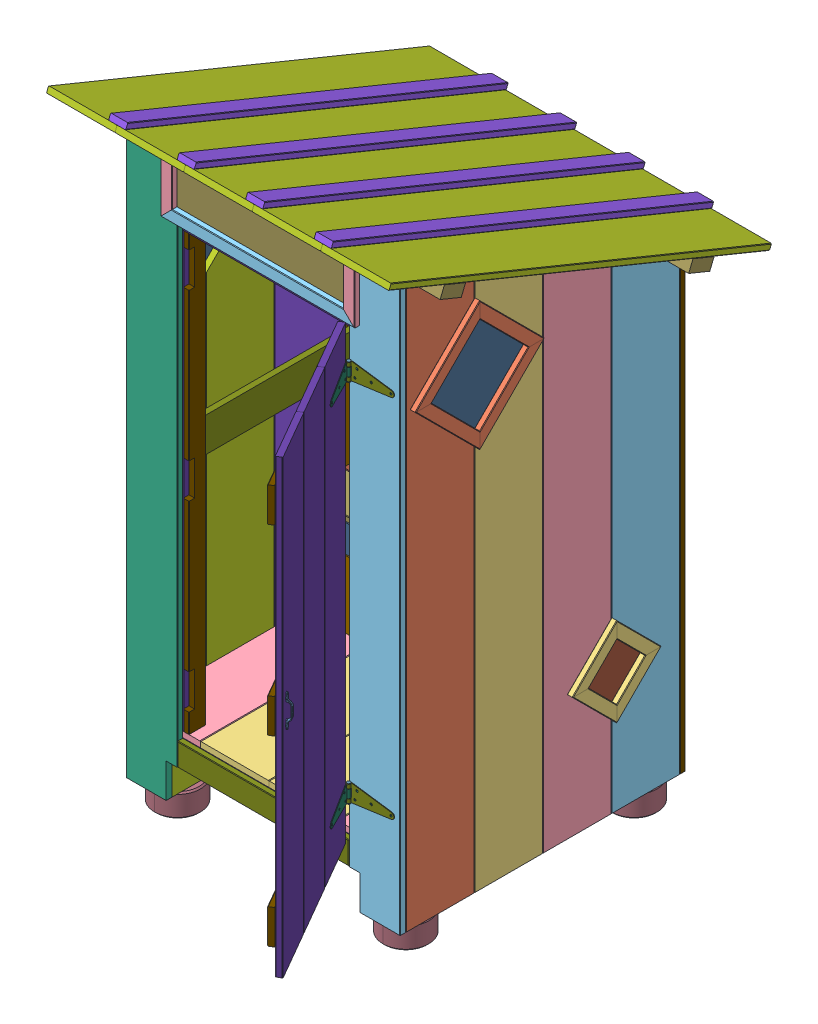
SolidWorks assembly Outhouse-Open, configuration Default. Lengths in mm.
Overall size (1695.08 2811.22 2224.36).
182 component instances, 68 part files, 0 mates.
Components (placement in the parent):
- Outhouse-Open.STEP-1: Outhouse-Open.STEP [Default] at (-818.6553 342.8748 -248.7995) size (1695.08 2811.22 2224.36)
  - Back Door.STEP-1: Back Door.STEP [Default] at (152.4 1042.8986 -654.4771) x (-1 0 0) z (0 -0.017452 0.999848) size (609.6 597.3 84.95)
    - Flat hinge_B-1078-15_ASM_D_faut.STEP-1: Flat hinge_B-1078-15_ASM_D_faut.STEP [Default] at (304.8 299.1 18.7) x (0 -1 0) z (-1 0 0) size (36.2 12.63 94.6)
      - Flat hinge 60 x 90_M.STEP-1: Flat hinge 60 x 90_M.STEP [Default] at origin size (36 12 90)
      - Flat hinge 60 x 90 PIN_D_faut.STEP-1: Flat hinge 60 x 90 PIN_D_faut.STEP [Default] at origin size (7.8 7.8 94.6)
      - Flat hinge 60 x 90_F.STEP-1: Flat hinge 60 x 90_F.STEP [Default] x (0.999848 -0.017452 0) z (0 0 -1) size (36 12 90)
    - Flat hinge_B-1078-15_ASM_D_faut-1.STEP-1: Flat hinge_B-1078-15_ASM_D_faut-1.STEP [Default] at (0 299.1 18.7) x (0 -1 0) z (-1 0 0) size (36.2 12.63 94.6)
      - Flat hinge 60 x 90_M.STEP-1: Flat hinge 60 x 90_M.STEP [Default] at origin size (36 12 90)
      - Flat hinge 60 x 90 PIN_D_faut.STEP-1: Flat hinge 60 x 90 PIN_D_faut.STEP [Default] at origin size (7.8 7.8 94.6)
      - Flat hinge 60 x 90_F.STEP-1: Flat hinge 60 x 90_F.STEP [Default] x (0.999848 -0.017452 0) z (0 0 -1) size (36 12 90)
    - cc2.STEP-1: cc2.STEP [Default] at origin size (304.8 584.2 25.4)
    - cc2.STEP-2: cc2.STEP [Default] at (304.8 0 0) size (304.8 584.2 25.4)
    - BDC.STEP-1: BDC.STEP [Default] at (152.4 215.9 -25.4) size (609.6 76.2 25.4)
    - BDC.STEP-2: BDC.STEP [Default] at (152.4 -114.3 -25.4) size (609.6 76.2 25.4)
    - 90031A247_PHILLIPS FLAT HEAD SCREWS FOR WOOD_90031A247.STEP-1: 90031A247_PHILLIPS FLAT HEAD SCREWS FOR WOOD_90031A247.STEP [Default] at (-29.5 280.1 3) x (0 0 -1) z (1 0 0) size (25.4 9.78 9.78)
    - 90031A247_PHILLIPS FLAT HEAD SCREWS FOR WOOD_90031A247.STEP-2: 90031A247_PHILLIPS FLAT HEAD SCREWS FOR WOOD_90031A247.STEP [Default] at (0 280.1 3) x (0 0 -1) z (1 0 0) size (25.4 9.78 9.78)
    - 90031A247_PHILLIPS FLAT HEAD SCREWS FOR WOOD_90031A247.STEP-3: 90031A247_PHILLIPS FLAT HEAD SCREWS FOR WOOD_90031A247.STEP [Default] at (29.5 280.1 3) x (0 0 -1) z (1 0 0) size (25.4 9.78 9.78)
    - 90031A247_PHILLIPS FLAT HEAD SCREWS FOR WOOD_90031A247.STEP-4: 90031A247_PHILLIPS FLAT HEAD SCREWS FOR WOOD_90031A247.STEP [Default] at (-29.5 279.8289 34.066) x (0 -0.017452 0.999848) z (0.99997 0.007739 0.000135) size (25.4 9.78 9.78)
    - 90031A247_PHILLIPS FLAT HEAD SCREWS FOR WOOD_90031A247.STEP-5: 90031A247_PHILLIPS FLAT HEAD SCREWS FOR WOOD_90031A247.STEP [Default] at (0 279.8289 34.066) x (0 -0.017452 0.999848) z (0.99997 0.007739 0.000135) size (25.4 9.78 9.78)
    - 90031A247_PHILLIPS FLAT HEAD SCREWS FOR WOOD_90031A247.STEP-6: 90031A247_PHILLIPS FLAT HEAD SCREWS FOR WOOD_90031A247.STEP [Default] at (29.5 279.8289 34.066) x (0 -0.017452 0.999848) z (0.99997 0.007739 0.000135) size (25.4 9.78 9.78)
    - 90031A247_PHILLIPS FLAT HEAD SCREWS FOR WOOD_90031A247.STEP-7: 90031A247_PHILLIPS FLAT HEAD SCREWS FOR WOOD_90031A247.STEP [Default] at (275.3 279.8289 34.066) x (0 -0.017452 0.999848) z (0.99997 0.007739 0.000135) size (25.4 9.78 9.78)
    - 90031A247_PHILLIPS FLAT HEAD SCREWS FOR WOOD_90031A247.STEP-8: 90031A247_PHILLIPS FLAT HEAD SCREWS FOR WOOD_90031A247.STEP [Default] at (304.8 279.8289 34.066) x (0 -0.017452 0.999848) z (0.99997 0.007739 0.000135) size (25.4 9.78 9.78)
    - 90031A247_PHILLIPS FLAT HEAD SCREWS FOR WOOD_90031A247.STEP-9: 90031A247_PHILLIPS FLAT HEAD SCREWS FOR WOOD_90031A247.STEP [Default] at (334.3 279.8289 34.066) x (0 -0.017452 0.999848) z (0.99997 0.007739 0.000135) size (25.4 9.78 9.78)
    - 90031A247_PHILLIPS FLAT HEAD SCREWS FOR WOOD_90031A247.STEP-10: 90031A247_PHILLIPS FLAT HEAD SCREWS FOR WOOD_90031A247.STEP [Default] at (275.3 280.1 3) x (0 0 -1) z (1 0 0) size (25.4 9.78 9.78)
    - 90031A247_PHILLIPS FLAT HEAD SCREWS FOR WOOD_90031A247.STEP-11: 90031A247_PHILLIPS FLAT HEAD SCREWS FOR WOOD_90031A247.STEP [Default] at (304.8 280.1 3) x (0 0 -1) z (1 0 0) size (25.4 9.78 9.78)
    - 90031A247_PHILLIPS FLAT HEAD SCREWS FOR WOOD_90031A247.STEP-12: 90031A247_PHILLIPS FLAT HEAD SCREWS FOR WOOD_90031A247.STEP [Default] at (334.3 280.1 3) x (0 0 -1) z (1 0 0) size (25.4 9.78 9.78)
  - Cover (k).STEP-1: Cover (k).STEP [Default] at (0 963.1186 -515.8179) x (1 0 0) z (0 0.996195 0.087156) size (508 75.94 423.22)
    - Flat hinge_B-1078-15_ASM_D_faut-2.STEP-1: Flat hinge_B-1078-15_ASM_D_faut-2.STEP [Default] at (-158.2 18.7 -197.5) x (0 0 1) z (-1 0 0) size (38.59 36.91 94.6)
      - Flat hinge 60 x 90_M.STEP-1: Flat hinge 60 x 90_M.STEP [Default] at origin size (36 12 90)
      - Flat hinge 60 x 90 PIN_D_faut.STEP-1: Flat hinge 60 x 90 PIN_D_faut.STEP [Default] at origin size (7.8 7.8 94.6)
      - Flat hinge 60 x 90_F.STEP-1: Flat hinge 60 x 90_F.STEP [Default] x (-0.087156 0.996195 0) z (0 0 -1) size (36 12 90)
    - Flat hinge_B-1078-15_ASM_D_faut-3.STEP-1: Flat hinge_B-1078-15_ASM_D_faut-3.STEP [Default] at (158.2 18.7 -197.5) x (0 0 1) z (-1 0 0) size (38.59 36.91 94.6)
      - Flat hinge 60 x 90_M.STEP-1: Flat hinge 60 x 90_M.STEP [Default] at origin size (36 12 90)
      - Flat hinge 60 x 90 PIN_D_faut.STEP-1: Flat hinge 60 x 90 PIN_D_faut.STEP [Default] at origin size (7.8 7.8 94.6)
      - Flat hinge 60 x 90_F.STEP-1: Flat hinge 60 x 90_F.STEP [Default] x (-0.087156 0.996195 0) z (0 0 -1) size (36 12 90)
    - kk.STEP-1: kk.STEP [Default] at origin size (508 25.4 381)
    - kkC.STEP-1: kkC.STEP [Default] at (-228.6 25.4 0) size (50.8 25.4 381)
    - kkC.STEP-2: kkC.STEP [Default] at (228.6 25.4 0) size (50.8 25.4 381)
    - kkk.STEP-1: kkk.STEP [Default] at (0 36.8347 -217.858) x (0 0.996195 -0.087156) z (1 0 0) size (50.8 25.4 508)
  - 10 Gal w lid - 6110.STEP-1: 10 Gal w lid - 6110.STEP [Default] at (0 279.654 -368.3) size (438.15 387.86 414.11)
    - PAIL^10 Gal w lid - 6110.STEP-1: PAIL^10 Gal w lid - 6110.STEP [Default] at origin size (427.62 387.86 400.56)
      - PAIL^PAIL_10 Gal w lid - 6110.STEP-1: PAIL^PAIL_10 Gal w lid - 6110.STEP [Default] at origin size (427.62 387.86 400.56)
    - WIRE HANDLE^10 Gal w lid - 6110(01).STEP-1: WIRE HANDLE^10 Gal w lid - 6110(01).STEP [Default] at (0 438.4989 258.0888) x (1 0 0) z (0 0.866025 -0.5) size (438.15 258.31 28.95)
  - Tower Bolt Lock.STEP-1: Tower Bolt Lock.STEP [Default] at (-345.939 249.688 -622.8267) x (0 -1 0) z (1 0 0) size (55.55 20.7 100)
    - Tower Bolt Lock A.STEP-1: Tower Bolt Lock A.STEP [Default] at (-1014.0808 5.0917 43.679) x (-0.999848 -0.017452 0) z (0 0 1) size (40 20 100)
    - Tower Bolt Lock C.STEP-1: Tower Bolt Lock C.STEP [Default] at (-1014.0808 5.0917 43.679) x (0.997928 -0.064342 0) z (0 0 1) size (42 14 100)
  - Front Door.STEP-1: Front Door.STEP [Default] at (438.148 1257.3 769.6836) x (-0.5 0 -0.866025) z (0.866025 0 -0.5) size (787.38 2006.6 265.05)
    - STRAP HINGE.STEP-1: STRAP HINGE.STEP [Default] at (140.6804 642.3442 45.0071) x (-0.387214 0 0.92199) z (-0.92199 0 -0.387214) size (205.92 79.31 194.19)
      - SH3.STEP-1: SH3.STEP [Default] at origin size (15.51 79.31 15.51)
      - SH1.STEP-1: SH1.STEP [Default] at (-42.0217 0 2.0112) x (-0.387214 0 -0.92199) z (0.92199 0 -0.387214) size (204.1 74.69 15.51)
      - SH2.STEP-1: SH2.STEP [Default] at (1.7199 0 2.6749) x (0.992074 0 0.125658) z (-0.125658 0 0.992074) size (204.1 76.2 15.51)
    - STRAP HINGE-1.STEP-1: STRAP HINGE-1.STEP [Default] at (140.6804 -983.2558 45.0071) x (-0.387214 0 0.92199) z (-0.92199 0 -0.387214) size (205.92 79.31 194.19)
      - SH3.STEP-1: SH3.STEP [Default] at origin size (15.51 79.31 15.51)
      - SH1.STEP-1: SH1.STEP [Default] at (-42.0217 0 2.0112) x (-0.387214 0 -0.92199) z (0.92199 0 -0.387214) size (204.1 74.69 15.51)
      - SH2.STEP-1: SH2.STEP [Default] at (1.7199 0 2.6749) x (0.992074 0 0.125658) z (-0.125658 0 0.992074) size (204.1 76.2 15.51)
    - qq.STEP-1: qq.STEP [Default] at origin size (254 2006.6 25.4)
    - qq.STEP-2: qq.STEP [Default] at (-254 0 0) size (254 2006.6 25.4)
    - qq.STEP-3: qq.STEP [Default] at (-508 0 0) size (254 2006.6 25.4)
    - pp.STEP-1: pp.STEP [Default] at (-254 0 -25.4) size (762 152.4 25.4)
    - pp.STEP-2: pp.STEP [Default] at (-254 -812.8 -25.4) size (762 152.4 25.4)
    - pp.STEP-3: pp.STEP [Default] at (-254 812.8 -25.4) size (762 152.4 25.4)
    - 20022.STEP-1: 20022.STEP [Default] at (-584.2 -72.5805 12.7) x (1 0 0) z (0 -1 0) size (18.35 21.9 145.16)
    - 90031A247_PHILLIPS FLAT HEAD SCREWS FOR WOOD_90031A247.STEP-1: 90031A247_PHILLIPS FLAT HEAD SCREWS FOR WOOD_90031A247.STEP [Default] at (-47.8076 812.8 2.794) x (0 0 -1) z (1 0 0) size (25.4 9.78 9.78)
    - 90031A247_PHILLIPS FLAT HEAD SCREWS FOR WOOD_90031A247.STEP-2: 90031A247_PHILLIPS FLAT HEAD SCREWS FOR WOOD_90031A247.STEP [Default] at (39.5049 812.8 2.794) x (0 0 -1) z (1 0 0) size (25.4 9.78 9.78)
    - 90031A247_PHILLIPS FLAT HEAD SCREWS FOR WOOD_90031A247.STEP-3: 90031A247_PHILLIPS FLAT HEAD SCREWS FOR WOOD_90031A247.STEP [Default] at (103.0049 832.6438 2.794) x (0 0 -1) z (1 0 0) size (25.4 9.78 9.78)
    - 90031A247_PHILLIPS FLAT HEAD SCREWS FOR WOOD_90031A247.STEP-4: 90031A247_PHILLIPS FLAT HEAD SCREWS FOR WOOD_90031A247.STEP [Default] at (112.5299 793.75 2.794) x (0 0 -1) z (1 0 0) size (25.4 9.78 9.78)
    - 90031A247_PHILLIPS FLAT HEAD SCREWS FOR WOOD_90031A247.STEP-5: 90031A247_PHILLIPS FLAT HEAD SCREWS FOR WOOD_90031A247.STEP [Default] at (138.9373 793.75 48.5328) x (0.866025 0 0.5) z (-0.5 0 0.866025) size (25.4 9.78 9.78)
    - 90031A247_PHILLIPS FLAT HEAD SCREWS FOR WOOD_90031A247.STEP-6: 90031A247_PHILLIPS FLAT HEAD SCREWS FOR WOOD_90031A247.STEP [Default] at (134.1748 832.6438 56.7817) x (0.866025 0 0.5) z (-0.5 0 0.866025) size (25.4 9.78 9.78)
    - 90031A247_PHILLIPS FLAT HEAD SCREWS FOR WOOD_90031A247.STEP-7: 90031A247_PHILLIPS FLAT HEAD SCREWS FOR WOOD_90031A247.STEP [Default] at (102.4248 812.8 111.7743) x (0.866025 0 0.5) z (-0.5 0 0.866025) size (25.4 9.78 9.78)
    - 90031A247_PHILLIPS FLAT HEAD SCREWS FOR WOOD_90031A247.STEP-8: 90031A247_PHILLIPS FLAT HEAD SCREWS FOR WOOD_90031A247.STEP [Default] at (58.7685 812.8 187.3892) x (0.866025 0 0.5) z (-0.5 0 0.866025) size (25.4 9.78 9.78)
    - 90031A247_PHILLIPS FLAT HEAD SCREWS FOR WOOD_90031A247.STEP-9: 90031A247_PHILLIPS FLAT HEAD SCREWS FOR WOOD_90031A247.STEP [Default] at (-47.8076 -812.8 2.794) x (0 0 -1) z (1 0 0) size (25.4 9.78 9.78)
    - 90031A247_PHILLIPS FLAT HEAD SCREWS FOR WOOD_90031A247.STEP-10: 90031A247_PHILLIPS FLAT HEAD SCREWS FOR WOOD_90031A247.STEP [Default] at (39.5049 -812.8 2.794) x (0 0 -1) z (1 0 0) size (25.4 9.78 9.78)
    - 90031A247_PHILLIPS FLAT HEAD SCREWS FOR WOOD_90031A247.STEP-11: 90031A247_PHILLIPS FLAT HEAD SCREWS FOR WOOD_90031A247.STEP [Default] at (112.5299 -831.85 2.794) x (0 0 -1) z (1 0 0) size (25.4 9.78 9.78)
    - 90031A247_PHILLIPS FLAT HEAD SCREWS FOR WOOD_90031A247.STEP-12: 90031A247_PHILLIPS FLAT HEAD SCREWS FOR WOOD_90031A247.STEP [Default] at (103.0049 -792.9563 2.794) x (0 0 -1) z (1 0 0) size (25.4 9.78 9.78)
    - 90031A247_PHILLIPS FLAT HEAD SCREWS FOR WOOD_90031A247.STEP-13: 90031A247_PHILLIPS FLAT HEAD SCREWS FOR WOOD_90031A247.STEP [Default] at (138.9373 -831.85 48.5328) x (0.866025 0 0.5) z (-0.5 0 0.866025) size (25.4 9.78 9.78)
    - 90031A247_PHILLIPS FLAT HEAD SCREWS FOR WOOD_90031A247.STEP-14: 90031A247_PHILLIPS FLAT HEAD SCREWS FOR WOOD_90031A247.STEP [Default] at (134.1748 -792.9563 56.7817) x (0.866025 0 0.5) z (-0.5 0 0.866025) size (25.4 9.78 9.78)
    - 90031A247_PHILLIPS FLAT HEAD SCREWS FOR WOOD_90031A247.STEP-15: 90031A247_PHILLIPS FLAT HEAD SCREWS FOR WOOD_90031A247.STEP [Default] at (102.4248 -812.8 111.7743) x (0.866025 0 0.5) z (-0.5 0 0.866025) size (25.4 9.78 9.78)
    - 90031A247_PHILLIPS FLAT HEAD SCREWS FOR WOOD_90031A247.STEP-16: 90031A247_PHILLIPS FLAT HEAD SCREWS FOR WOOD_90031A247.STEP [Default] at (58.7685 -812.8 187.3892) x (0.866025 0 0.5) z (-0.5 0 0.866025) size (25.4 9.78 9.78)
  - WAl.STEP-1: WAl.STEP [Default] at (622.3 2132.3236 430.5236) x (0 -0.707107 -0.707107) z (0 -0.707107 0.707107) size (406.4 25.4 406.4)
    - WAl-0.STEP-1: WAl-0.STEP [Default] at origin size (50.8 25.4 406.4)
    - WAl-0.STEP-2: WAl-0.STEP [Default] at (177.8 0 177.8) x (0 0 -1) z (1 0 0) size (50.8 25.4 406.4)
    - WAl-0.STEP-3: WAl-0.STEP [Default] at (355.6 0 0) x (-1 0 0) z (0 0 -1) size (50.8 25.4 406.4)
    - WAl-0.STEP-4: WAl-0.STEP [Default] at (177.8 0 -177.8) x (0 0 1) z (-1 0 0) size (50.8 25.4 406.4)
  - WBl.STEP-1: WBl.STEP [Default] at (622.3 639.6223 -223.9777) x (0 -0.707107 -0.707107) z (0 -0.707107 0.707107) size (279.4 25.4 279.4)
    - WBl-1.STEP-1: WBl-1.STEP [Default] at origin size (50.8 25.4 279.4)
    - WBl-1.STEP-2: WBl-1.STEP [Default] at (114.3 0 114.3) x (0 0 -1) z (1 0 0) size (50.8 25.4 279.4)
    - WBl-1.STEP-3: WBl-1.STEP [Default] at (228.6 0 0) x (-1 0 0) z (0 0 -1) size (50.8 25.4 279.4)
    - WBl-1.STEP-4: WBl-1.STEP [Default] at (114.3 0 -114.3) x (0 0 1) z (-1 0 0) size (50.8 25.4 279.4)
  - WBl-1-2.STEP-1: WBl-1-2.STEP [Default] at (-622.3 477.9777 -385.6223) x (0 0.707107 0.707107) z (0 -0.707107 0.707107) size (279.4 25.4 279.4)
    - WBl-1.STEP-1: WBl-1.STEP [Default] at origin size (50.8 25.4 279.4)
    - WBl-1.STEP-2: WBl-1.STEP [Default] at (114.3 0 114.3) x (0 0 -1) z (1 0 0) size (50.8 25.4 279.4)
    - WBl-1.STEP-3: WBl-1.STEP [Default] at (228.6 0 0) x (-1 0 0) z (0 0 -1) size (50.8 25.4 279.4)
    - WBl-1.STEP-4: WBl-1.STEP [Default] at (114.3 0 -114.3) x (0 0 1) z (-1 0 0) size (50.8 25.4 279.4)
  - WAl-1.STEP-1: WAl-1.STEP [Default] at (-622.3 1880.8764 179.0764) x (0 0.707107 0.707107) z (0 -0.707107 0.707107) size (406.4 25.4 406.4)
    - WAl-0.STEP-1: WAl-0.STEP [Default] at origin size (50.8 25.4 406.4)
    - WAl-0.STEP-2: WAl-0.STEP [Default] at (177.8 0 177.8) x (0 0 -1) z (1 0 0) size (50.8 25.4 406.4)
    - WAl-0.STEP-3: WAl-0.STEP [Default] at (355.6 0 0) x (-1 0 0) z (0 0 -1) size (50.8 25.4 406.4)
    - WAl-0.STEP-4: WAl-0.STEP [Default] at (177.8 0 -177.8) x (0 0 1) z (-1 0 0) size (50.8 25.4 406.4)
  - WCl.STEP-1: WCl.STEP [Default] at (-406.4 2416.175 647.7) x (1 0 0) z (0 -1 0) size (863.6 25.4 304.8)
    - WCl1.STEP-1: WCl1.STEP [Default] at origin size (50.8 25.4 304.8)
    - WCl1.STEP-2: WCl1.STEP [Default] at (812.8 0 0) x (-1 0 0) z (0 0 -1) size (50.8 25.4 304.8)
    - WCl2.STEP-1: WCl2.STEP [Default] at (406.4 0 -127) x (0 0 1) z (-1 0 0) size (50.8 25.4 863.6)
    - WCl2.STEP-2: WCl2.STEP [Default] at (406.4 0 127) x (0 0 -1) z (1 0 0) size (50.8 25.4 863.6)
  - B.STEP-1: B.STEP [Default] at (0 203.2 0) x (0 0 -1) z (1 0 0) size (101.6 101.6 1168.4)
  - A.STEP-1: A.STEP [Default] at (508 76.2 0) size (152.4 152.4 1219.2)
  - C.STEP-1: C.STEP [Default] at (0 203.2 558.8) x (0 0 -1) z (1 0 0) size (101.6 101.6 1016)
  - C.STEP-2: C.STEP [Default] at (0 203.2 -558.8) x (0 0 -1) z (1 0 0) size (101.6 101.6 1016)
  - D.STEP-1: D.STEP [Default] at (533.4 1333.5 558.8) x (1 0 0) z (0 -1 0) size (50.8 101.6 2362.2)
  - E.STEP-1: E.STEP [Default] at (431.8 1231.9 558.8) x (1 0 0) z (0 -1 0) size (50.8 101.6 1955.8)
  - F.STEP-1: F.STEP [Default] at (533.4 1104.9 -558.8) x (1 0 0) z (0 -1 0) size (50.8 101.6 1905)
  - G.STEP-1: G.STEP [Default] at (0 2066.4478 -552.9649) x (0 0.925541 -0.378649) z (-1 0 0) size (50.8 101.6 1524)
  - G.STEP-2: G.STEP [Default] at (0 2518.8734 552.9649) x (0 0.925541 -0.378649) z (-1 0 0) size (50.8 101.6 1524)
  - K.STEP-1: K.STEP [Default] at (571.5 2179.5982 -8.0427) x (0 -0.925547 0.378633) z (0 0.378633 0.925547) size (152.4 25.4 1379.62)
  - H.STEP-1: H.STEP [Default] at (0 2273.6338 -46.5118) x (0 0.925547 -0.378633) z (1 0 0) size (50.8 101.6 1168.4)
  - J.STEP-1: J.STEP [Default] at (482.6 1231.9 558.8) x (1 0 0) z (0 -1 0) size (50.8 101.6 76.2)
  - L.STEP-1: L.STEP [Default] at (571.5 1193.8 0) x (0 -1 0) z (0 0 1) size (152.4 25.4 1219.2)
  - A.STEP-2: A.STEP [Default] at (-508 76.2 0) x (-1 0 0) z (0 0 -1) size (152.4 152.4 1219.2)
  - D.STEP-2: D.STEP [Default] at (-533.4 1333.5 558.8) x (1 0 0) z (0 -1 0) size (50.8 101.6 2362.2)
  - E.STEP-2: E.STEP [Default] at (-431.8 1231.9 558.8) x (-1 0 0) z (0 1 0) size (50.8 101.6 1955.8)
  - F.STEP-2: F.STEP [Default] at (-533.4 1104.9 -558.8) x (1 0 0) z (0 -1 0) size (50.8 101.6 1905)
  - J.STEP-2: J.STEP [Default] at (-482.6 1231.9 558.8) x (-1 0 0) z (0 1 0) size (50.8 101.6 76.2)
  - L.STEP-2: L.STEP [Default] at (-571.5 1193.8 0) x (0 -1 0) z (0 0 -1) size (152.4 25.4 1219.2)
  - K.STEP-2: K.STEP [Default] at (-571.5 2179.5982 -8.0427) x (0 -0.925547 0.378633) z (0 0.378633 0.925547) size (152.4 25.4 1379.62)
  - I.STEP-1: I.STEP [Default] at (0 2235.2 558.8) x (0 1 0) z (1 0 0) size (50.8 101.6 1016)
  - I.STEP-2: I.STEP [Default] at (0 1498.6 -558.8) x (0 1 0) z (1 0 0) size (50.8 101.6 1016)
  - bb.STEP-1: bb.STEP [Default] at (457.2 1031.875 -622.3) size (304.8 2063.75 25.4)
  - cc1.STEP-1: cc1.STEP [Default] at (152.4 1400.175 -622.3) size (304.8 1327.15 25.4)
  - bb-3.STEP-1: bb-3.STEP [Default] at (-457.2 1031.875 -622.3) x (-1 0 0) z (0 0 -1) size (304.8 2063.75 25.4)
  - cc1.STEP-2: cc1.STEP [Default] at (-152.4 1400.175 -622.3) x (-1 0 0) z (0 0 -1) size (304.8 1327.15 25.4)
  - dd.STEP-1: dd.STEP [Default] at (152.4 266.7 0) size (304.8 25.4 1219.2)
  - dd1.STEP-1: dd1.STEP [Default] at (444.5 266.7 0) size (279.4 25.4 1219.2)
  - dd.STEP-2: dd.STEP [Default] at (-152.4 266.7 0) x (-1 0 0) z (0 0 -1) size (304.8 25.4 1219.2)
  - dd1.STEP-2: dd1.STEP [Default] at (-444.5 266.7 0) x (-1 0 0) z (0 0 1) size (279.4 25.4 1219.2)
  - ccc.STEP-1: ccc.STEP [Default] at (495.3 1284.2875 622.3) size (228.6 2568.58 25.4)
  - ccc-4.STEP-1: ccc-4.STEP [Default] at (-495.3 1284.2875 622.3) x (-1 0 0) z (0 0 -1) size (228.6 2568.58 25.4)
  - ff.STEP-1: ff.STEP [Default] at (609.6 2328.1317 -13.9199) x (1 0 0) z (0 -0.925547 0.378633) size (304.8 1828.8 25.4)
  - ff.STEP-2: ff.STEP [Default] at (304.8 2328.1317 -13.9199) x (1 0 0) z (0 -0.925547 0.378633) size (304.8 1828.8 25.4)
  - ff.STEP-3: ff.STEP [Default] at (0 2328.1317 -13.9199) x (1 0 0) z (0 -0.925547 0.378633) size (304.8 1828.8 25.4)
  - ff.STEP-4: ff.STEP [Default] at (-304.8 2328.1317 -13.9199) x (-1 0 0) z (0 0.925547 -0.378633) size (304.8 1828.8 25.4)
  - ff.STEP-5: ff.STEP [Default] at (-609.6 2328.1317 -13.9199) x (-1 0 0) z (0 0.925547 -0.378633) size (304.8 1828.8 25.4)
  - ffl.STEP-1: ffl.STEP [Default] at (457.2 2351.6406 -23.5372) x (1 0 0) z (0 0.378633 0.925547) size (76.2 25.4 1828.8)
  - ffl.STEP-2: ffl.STEP [Default] at (152.4 2351.6406 -23.5372) x (1 0 0) z (0 0.378633 0.925547) size (76.2 25.4 1828.8)
  - ffl.STEP-3: ffl.STEP [Default] at (-152.4 2351.6406 -23.5372) x (1 0 0) z (0 0.378633 0.925547) size (76.2 25.4 1828.8)
  - ffl.STEP-4: ffl.STEP [Default] at (-457.2 2351.6406 -23.5372) x (1 0 0) z (0 0.378633 0.925547) size (76.2 25.4 1828.8)
  - gg.STEP-1: gg.STEP [Default] at (0 431.8 -139.7) x (0 1 0) z (0 0 1) size (304.8 1168.4 25.4)
  - hh.STEP-1: hh.STEP [Default] at (0 647.7 -139.7) x (0 -1 0) z (0 0 1) size (127 1168.4 25.4)
  - ii.STEP-1: ii.STEP [Default] at (0 723.9 -457.2) x (0 0 1) z (0 -1 0) size (312.79 1168.4 25.4)
  - jj.STEP-1: jj.STEP [Default] at (0 723.9 -215.9) x (0 0 1) z (0 -1 0) size (181.41 1168.4 25.4)
  - ll.STEP-1: ll.STEP [Default] at (0 1117.6 -565.15) size (50.8 152.4 88.9)
  - nn.STEP-1: nn.STEP [Default] at (196.6382 292.1 -308.6401) x (-0.34202 0 0.939693) z (0 1 0) size (304.8 76.2 25.4)
  - nn.STEP-2: nn.STEP [Default] at (-196.6382 292.1 -308.6401) x (0.34202 0 0.939693) z (0 -1 0) size (304.8 76.2 25.4)
  - Tower Bolt Lock B.STEP-1: Tower Bolt Lock B.STEP [Default] at (-337.34 223.2 -645) x (0 -1 0) z (1 0 0) size (40 20 30)
  - rr.STEP-1: rr.STEP [Default] at (0 203.2 622.3) x (0 -1 0) z (0 0 1) size (101.6 762 25.4)
  - ss.STEP-1: ss.STEP [Default] at (-393.7 1244.6 571.5) x (0 1 0) z (-1 0 0) size (1930.4 76.2 25.4)
  - ss-5.STEP-1: ss-5.STEP [Default] at (-368.3 1244.6 571.5) x (0 1 0) z (-1 0 0) size (1930.4 76.2 25.4)
  - vv.STEP-1: vv.STEP [Default] at (0 2273.3 609.6) x (0 0 -1) z (0 -1 0) size (50.8 762 25.4)
  - vv.STEP-2: vv.STEP [Default] at (0 2543.175 622.3) x (0 1 0) z (0 0 -1) size (50.8 762 25.4)
  - aa.STEP-1: aa.STEP [Default] at (596.9 1282.7 457.2) x (0 0 1) z (-1 0 0) size (304.8 2565.4 25.4)
  - aa-6.STEP-1: aa-6.STEP [Default] at (596.9 1282.7 152.4) x (0 0 1) z (-1 0 0) size (304.8 2444.8 25.4)
  - aa-7.STEP-1: aa-7.STEP [Default] at (596.9 1282.7 -152.4) x (0 0 1) z (-1 0 0) size (304.8 2320.1 25.4)
  - aa-8.STEP-1: aa-8.STEP [Default] at (596.9 1282.7 -457.2) x (0 0 1) z (-1 0 0) size (304.8 2195.41 25.4)
  - aa-9.STEP-1: aa-9.STEP [Default] at (-596.9 1282.7 457.2) x (0 0 1) z (-1 0 0) size (304.8 2565.4 25.4)
  - aa-10.STEP-1: aa-10.STEP [Default] at (-596.9 1282.7 152.4) x (0 0 1) z (-1 0 0) size (304.8 2444.8 25.4)
  - aa-11.STEP-1: aa-11.STEP [Default] at (-596.9 1282.7 -152.4) x (0 0 1) z (-1 0 0) size (304.8 2320.1 25.4)
  - aa-12.STEP-1: aa-12.STEP [Default] at (-596.9 1282.7 -457.2) x (0 0 1) z (-1 0 0) size (304.8 2195.41 25.4)
  - Mesh-A.STEP-1: Mesh-A.STEP [Default] at (609.6 2006.6 304.8) size (0.76 502.89 502.89)
  - Mesh-B.STEP-1: Mesh-B.STEP [Default] at (609.6 558.8 -304.8) size (0.76 323.29 323.29)
  - Mesh-B.STEP-2: Mesh-B.STEP [Default] at (-609.6 558.8 -304.8) x (-1 0 0) z (0 0 -1) size (0.76 323.29 323.29)
  - Mesh-A.STEP-2: Mesh-A.STEP [Default] at (-609.6 2006.6 304.8) x (-1 0 0) z (0 0 -1) size (0.76 502.89 502.89)
  - Mesh-C.STEP-1: Mesh-C.STEP [Default] at (0 2403.475 635) x (0 0 1) z (-1 0 0) size (0.76 279.4 812.8)
  - Paver.STEP-1: Paver.STEP [Default] at (508 -101.6 508) size (203.2 101.6 203.2)
  - Paver.STEP-2: Paver.STEP [Default] at (508 -101.6 -508) size (203.2 101.6 203.2)
  - Paver.STEP-3: Paver.STEP [Default] at (-508 -101.6 508) x (-1 0 0) z (0 0 -1) size (203.2 101.6 203.2)
  - Paver.STEP-4: Paver.STEP [Default] at (-508 -101.6 -508) x (-1 0 0) z (0 0 -1) size (203.2 101.6 203.2)
  - 90031A133_PHILLIPS FLAT HEAD SCREWS FOR WOOD_90031A133.STEP-1: 90031A133_PHILLIPS FLAT HEAD SCREWS FOR WOOD_90031A133.STEP [Default] at (-212.26 1249.1149 -647.8772) x (0 0.017452 -0.999848) z (-1 0 0) size (25.4 6.4 6.4)
  - 90031A133_PHILLIPS FLAT HEAD SCREWS FOR WOOD_90031A133.STEP-2: 90031A133_PHILLIPS FLAT HEAD SCREWS FOR WOOD_90031A133.STEP [Default] at (-212.26 1279.1103 -647.3536) x (0 0.017452 -0.999848) z (-1 0 0) size (25.4 6.4 6.4)
  - 90031A133_PHILLIPS FLAT HEAD SCREWS FOR WOOD_90031A133.STEP-3: 90031A133_PHILLIPS FLAT HEAD SCREWS FOR WOOD_90031A133.STEP [Default] at (-292.26 1249.1149 -647.8772) x (0 0.017452 -0.999848) z (-1 0 0) size (25.4 6.4 6.4)
  - 90031A133_PHILLIPS FLAT HEAD SCREWS FOR WOOD_90031A133.STEP-4: 90031A133_PHILLIPS FLAT HEAD SCREWS FOR WOOD_90031A133.STEP [Default] at (-292.26 1279.1103 -647.3536) x (0 0.017452 -0.999848) z (-1 0 0) size (25.4 6.4 6.4)
  - 90031A133_PHILLIPS FLAT HEAD SCREWS FOR WOOD_90031A133.STEP-5: 90031A133_PHILLIPS FLAT HEAD SCREWS FOR WOOD_90031A133.STEP [Default] at (-314.84 238.2 -625.3) x (0 0 1) z (-1 0 0) size (25.4 6.4 6.4)
  - 90031A133_PHILLIPS FLAT HEAD SCREWS FOR WOOD_90031A133.STEP-6: 90031A133_PHILLIPS FLAT HEAD SCREWS FOR WOOD_90031A133.STEP [Default] at (-329.84 238.2 -625.3) x (0 0 1) z (-1 0 0) size (25.4 6.4 6.4)
  - 90031A133_PHILLIPS FLAT HEAD SCREWS FOR WOOD_90031A133.STEP-7: 90031A133_PHILLIPS FLAT HEAD SCREWS FOR WOOD_90031A133.STEP [Default] at (-314.84 208.2 -625.3) x (0 0 1) z (-1 0 0) size (25.4 6.4 6.4)
  - 90031A133_PHILLIPS FLAT HEAD SCREWS FOR WOOD_90031A133.STEP-8: 90031A133_PHILLIPS FLAT HEAD SCREWS FOR WOOD_90031A133.STEP [Default] at (-329.84 208.2 -625.3) x (0 0 1) z (-1 0 0) size (25.4 6.4 6.4)
